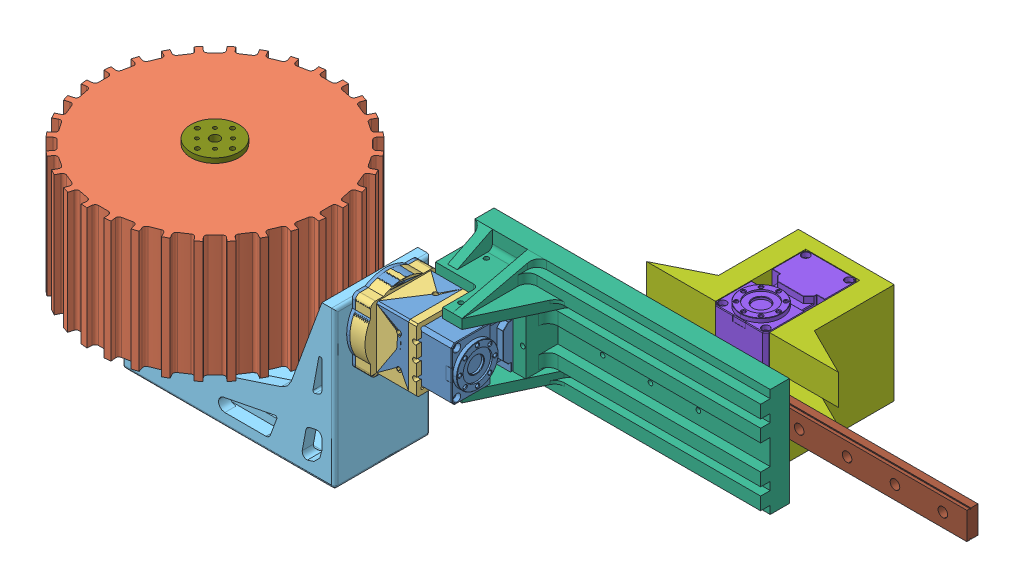
SolidWorks assembly 单轮, configuration Default. Lengths in mm.
Overall size (517.91 123.6 255.15).
20 component instances, 16 part files, 42 mates.
Components (placement in the parent):
- 540总装-1: 540总装 [默认] at (-9.2345 7.2685 42.6291) size (68.75 59.5 48)
- 透明车轮-加工版-1: 透明车轮-加工版 [默认] at (4.5155 78.2685 59.3791) x (0.707107 0 0.707107) z (0 -1 0) size (149.62 149.62 76)
- 3813d-00_asm-2.0-1: 3813d-00_asm-2.0 [默认] at (4.5155 -18.8315 59.3791) x (0.5 0 0.866025) z (0 -1 0)
- 外壳.step-1: 外壳.step [默认] at (-9.2345 51.2685 76.1291) x (0 0 -1) z (0 -1 0) size (48 48 34.5)
- 方案2-大L-1: 方案2-大L [Default] at (39.3905 4.6685 59.3791) x (0 0 -1) z (1 0 0) size (47.8 57 70.75)
- L连接-1: L连接 [Default] at (4.5155 -42.3315 29.3791) x (0 0 1) z (0 1 0) size (60 135 98)
- 540总装-2: 540总装 [默认] at (166.5155 23.5185 73.1291) x (0 0 -1) z (0 1 0) size (68.75 59.5 48)
- 外壳.step-2: 外壳.step [默认] at (122.5155 57.0185 73.1291) x (0 -1 0) z (1 0 0) size (48 48 34.5)
- 新的升降台v4-1: 新的升降台v4 [Default] at (307.5155 6.3685 2.6291) x (0 -1 0) z (0 0 1) size (67.8 185 66)
- 升降-1: 升降 [Default] at (303.824 125.8561 -95.2425) x (0 0 1) z (0 -1 0) size (74.21 120 65.6)
  - 板间外壳-1: 板间外壳 [Default] at (5.2631 83.2739 60.575) size (67 120 63.1)
  - 540舵机-1: 540舵机 [默认] at (58.5131 53.4239 82.575) x (0 -1 0) z (0 0 1) size (33.51 58.5 54.3)
  - 齿轮.step-1: 齿轮.step [默认] at (58.5131 53.4239 115.075) x (0 0 -1) z (-1 0.000114 0) size (8 41.91 41.91)
- HIWIN Corporation-MGW-9C-1: HIWIN Corporation-MGW-9C [Default] at (235.1626 45.0319 -5.4131) x (0 1 0) z (1 0 0) size (30 9.1 39.26)
- HIWIN Corporation-MGWR-9-R0500-1: HIWIN Corporation-MGWR-9-R0500 [Default] at (372.4175 47.7155 -2.8717) x (0 -1 0) z (-1 0 0) size (17 7 120)
- 齿条.step-1: 齿条.step [默认] at (201.2166 22.5685 10.7791) x (1 0 0) z (0 1 0) size (90 11 10)
- 三轴力传感器简易模型-1: 三轴力传感器简易模型 [默认] at (4.5155 -32.3315 59.3791) size (40 20 40)
- 相机固定件改-1: 相机固定件改 [默认] at (47.8155 23.1685 23.7791) x (0 -1 0) z (0 0 -1) size (43 21.7 40.2)
- 相机简易模型-1: 相机简易模型 [默认] at (25.5155 23.1685 21.2791) x (0 -1 0) z (0 0 -1) size (38.4 28.7 38.4)
- 轮子定位件-1: 轮子定位件 [默认] at (4.5155 64.4685 59.3791) x (1 0 0) z (0 1 0) size (30 30 16.8)
Mates (geometry in assembly coordinates):
- 同心1: concentric anti-aligned: cylinder of 540总装-1 through (4.5155 62.7685 59.3791) axis (0 -1 0) radius 16; cylinder of 透明车轮-加工版-1 through (4.5155 2.2685 59.3791) axis (0 1 0) radius 5.05
- 重合1: coincident anti-aligned: plane of 540总装-1 through (4.5155 64.2685 59.3791) normal (0 1 0); plane of 透明车轮-加工版-1 through (4.5155 64.2685 59.3791) normal (0 -1 0)
- 同心2: concentric anti-aligned: cylinder of 540总装-1 through (4.5155 7.3935 59.3791) axis (0 -1 0) radius 5; cylinder of 3813d-00_asm-2.0-1/3813d-00_asm.stp-1/3813D-00_ASM_99_ASM.stp-1/38133-27_40.stp-1 through (4.5155 -17.3315 59.3791) axis (0 1 0) radius 22.5
- 重合5: coincident aligned: plane of 540总装-1 through (-9.2345 51.2685 76.1291) normal (0 -1 0); plane of 外壳.step-1 through (-9.2345 51.2685 76.1291) normal (0 -1 0)
- 同心7: concentric aligned: cylinder of 540总装-1 through (4.5155 7.3935 59.3791) axis (0 -1 0) radius 5; circle of 外壳.step-1
- 同心11: concentric aligned: cylinder of 3813d-00_asm-2.0-1/3813d-00_asm.stp-1/3813D-00_ASM_99_ASM.stp-1/3813D-10_ASM_33_ASM.stp-1/3813D-15_181.stp-1 through (4.5155 -33.3315 59.3791) axis (0 1 0) radius 4.01; cylinder of 方案2-大L-1 through (4.5155 -3.3315 59.3791) axis (0 1 0) radius 4.125
- 同心12: concentric anti-aligned: cylinder of 3813d-00_asm-2.0-1/3813d-00_asm.stp-1/3813D-00_ASM_99_ASM.stp-1/3813D-10_ASM_33_ASM.stp-1/3813D-15_181.stp-1 through (12.5155 -21.7905 45.5227) axis (0 -1 0) radius 1.65; cylinder of 方案2-大L-1 through (12.5155 4.6685 45.5227) axis (0 1 0) radius 2.25
- 重合11: coincident anti-aligned: plane of 3813d-00_asm-2.0-1/3813d-00_asm.stp-1/3813D-00_ASM_99_ASM.stp-1/38133-29_43.stp-1 through (4.5155 -3.3315 59.3791) normal (0 1 0); plane of 方案2-大L-1 through (39.3905 -3.3315 59.3791) normal (0 -1 0)
- 平行4: parallel aligned: plane of 540总装-1 through (49.2655 7.2685 76.1291) normal (1 0 0); plane of 方案2-大L-1 through (53.2655 44.6685 59.3791) normal (1 0 0)
- 同心13: concentric aligned: cylinder of 540总装-1 through (42.5155 37.2685 72.3324) axis (0 0 -1) radius 1.025; cylinder of 方案2-大L-1 through (42.5155 37.2685 80.2791) axis (0 0 -1) radius 1.6
- 同心14: concentric aligned: cylinder of 540总装-1 through (10.5155 37.2685 79.1291) axis (0 0 -1) radius 1.5; cylinder of 外壳.step-1 through (10.5155 37.2685 79.1291) axis (0 0 -1) radius 1.5
- 同心15: concentric aligned: cylinder of 3813d-00_asm-2.0-1/3813d-00_asm.stp-1/3813D-00_ASM_99_ASM.stp-1/3813D-10_ASM_33_ASM.stp-1/3813D-15_181.stp-1 through (9.0155 -33.3315 67.1733) axis (0 1 0) radius 1.51; cylinder of 方案2-大L-1 through (-0.4845 -3.3315 64.3791) axis (0 1 0) radius 1.6
- 同心16: concentric aligned: cylinder of 3813d-00_asm-2.0-1/3813d-00_asm.stp-1/3813D-00_ASM_99_ASM.stp-1/3813D-26_48.stp-1 through (4.5155 -20.3315 59.3791) axis (0 -1 0) radius 22.5; cylinder of L连接-1 through (4.5155 -34.3315 59.3791) axis (0 -1 0) radius 30
- 重合12: coincident anti-aligned: plane of 3813d-00_asm-2.0-1/3813d-00_asm.stp-1/3813D-00_ASM_99_ASM.stp-1/38133-29_43.stp-2 through (4.5155 -34.3315 59.3791) normal (0 -1 0); plane of L连接-1 through (4.5155 -34.3315 29.3791) normal (0 1 0)
- 同心17: concentric anti-aligned: cylinder of 3813d-00_asm-2.0-1/3813d-00_asm.stp-1/3813D-00_ASM_99_ASM.stp-1/3813D-10_ASM_33_ASM.stp-1/3813D-15_181.stp-1 through (9.0155 -33.3315 67.1733) axis (0 1 0) radius 1.51; cylinder of L连接-1 through (9.0155 -34.3315 67.1733) axis (0 -1 0) radius 1.625
- 同心18: concentric aligned: cylinder of 540总装-2 through (109.5155 40.2685 59.3791) axis (1 0 0) radius 15; cylinder of 外壳.step-2 through (112.5155 40.2685 59.3791) axis (1 0 0) radius 14
- 重合13: coincident anti-aligned: plane of 540总装-2 through (122.5155 40.2685 59.3791) normal (-1 0 0); plane of 外壳.step-2 through (122.5155 57.0185 73.1291) normal (1 0 0)
- 同心19: concentric aligned: cylinder of 540总装-2 through (136.5155 30.2685 73.1291) axis (0 0 1) radius 1.5; cylinder of 外壳.step-2 through (136.5155 30.2685 73.1291) axis (0 0 1) radius 1.5
- 重合14: coincident anti-aligned: plane of L连接-1 through (109.5155 -34.3315 29.3791) normal (1 0 0); plane of 540总装-2 through (109.5155 40.2685 59.3791) normal (-1 0 0)
- 同心22: concentric anti-aligned: cylinder of L连接-1 through (39.5155 40.2685 59.3791) axis (1 0 0) radius 1.6; cylinder of 540总装-2 through (109.5155 40.2685 59.3791) axis (-1 0 0) radius 1.25
- 重合16: coincident anti-aligned: plane of 540总装-2 through (166.5155 57.0185 14.6291) normal (0 0 -1); plane of 新的升降台v4-1 through (307.5155 6.3685 14.6291) normal (0 0 1)
- 同心23: concentric anti-aligned: cylinder of 540总装-2 through (136.5155 50.2685 18.4258) axis (0 0 -1) radius 1.025; cylinder of 新的升降台v4-1 through (136.5155 50.2685 -1.4721) axis (0 0 1) radius 1.45
- 同心24: concentric anti-aligned: cylinder of 540总装-2 through (136.5155 30.2685 18.4258) axis (0 0 -1) radius 1.025; cylinder of 新的升降台v4-1 through (136.5155 30.2685 -1.4721) axis (0 0 1) radius 1.45
- 平行6: parallel aligned: plane of 新的升降台v4-1 through (307.5155 6.3685 2.6291) normal (0 0 -1); plane of L连接-1 through (4.5155 -34.3315 29.3791) normal (0 0 -1)
- 平行7: parallel anti-aligned: plane of 新的升降台v4-1 through (307.5155 6.3685 2.6291) normal (0 0 -1); plane of 升降-1/板间外壳-1 through (220.5501 21.1811 -24.9794) normal (0 0 1)
- 平行8: parallel aligned: plane of 新的升降台v4-1 through (307.5155 6.3685 14.6291) normal (1 0 0); plane of 升降-1/板间外壳-1 through (280.5501 21.1811 -89.9794) normal (1 0 0)
- 同心27: concentric anti-aligned: cylinder of HIWIN Corporation-MGW-9C-1 through (265.2255 39.4155 -1.5709) axis (-1 0 0) radius 0.35; cylinder of HIWIN Corporation-MGWR-9-R0500-1 through (122.4175 39.4155 -1.5709) axis (1 0 0) radius 0.35
- 重合20: coincident anti-aligned: plane of 新的升降台v4-1 through (307.5155 6.3685 10.7791) normal (0 0 -1); plane of 齿条.step-1 through (201.2166 12.5685 10.7791) normal (0 0 1)
- 重合22: coincident anti-aligned: plane of 新的升降台v4-1 through (307.5155 12.5685 10.7791) normal (0 1 0); plane of 齿条.step-1 through (201.2166 12.5685 -0.2209) normal (0 -1 0)
- 重合28: coincident anti-aligned: plane of 方案2-大L-1 through (27.5155 49.2689 45.4791) normal (-1 0 0); plane of 相机固定件改-1 through (27.5155 51.2343 45.2791) normal (1 0 0)
- 重合29: coincident aligned: plane of 方案2-大L-1 through (39.3905 44.6685 59.3791) normal (0 1 0); plane of 相机固定件改-1 through (23.8155 44.6685 2.2791) normal (0 1 0)
- 重合30: coincident aligned: plane of 方案2-大L-1 through (39.3905 44.6685 42.4791) normal (0 0 1); plane of 相机固定件改-1 through (33.8155 47.084 42.4791) normal (0 0 1)
- 重合31: coincident anti-aligned: plane of 相机固定件改-1 through (25.5155 23.1685 23.7791) normal (-1 0 0); plane of 相机简易模型-1 through (25.5155 23.1685 21.2791) normal (1 0 0)
- 同心29: concentric anti-aligned: circle of 相机固定件改-1; circle of 相机简易模型-1
- 平行13: parallel aligned: plane of 相机固定件改-1 through (23.8155 44.6685 2.2791) normal (0 0 -1); plane of 相机简易模型-1 through (23.8155 42.3685 2.0791) normal (0 0 -1)
- 同心30: concentric aligned: cylinder of 方案2-大L-1 through (-0.4845 -3.3315 54.3791) axis (0 1 0) radius 1.6; circle of 三轴力传感器简易模型-1
- 平行14: parallel aligned: plane of 方案2-大L-1 through (39.3905 4.6685 35.4791) normal (0 0 -1); plane of 三轴力传感器简易模型-1 through (-15.4845 -12.3315 39.3791) normal (0 0 -1)
- 重合33: coincident anti-aligned: plane of L连接-1 through (4.5155 -32.3315 29.3791) normal (0 1 0); plane of 三轴力传感器简易模型-1 through (4.5155 -32.3315 59.3791) normal (0 -1 0)
- 同心31: concentric anti-aligned: cylinder of 540总装-1 through (4.5155 64.2685 48.3791) axis (0 1 0) radius 1.45; cylinder of 透明车轮-加工版-1 through (4.5155 78.2685 48.3791) axis (0 -1 0) radius 1.45
- 重合34: coincident anti-aligned: plane of 透明车轮-加工版-1 through (4.5155 78.2685 59.3791) normal (0 1 0); plane of 轮子定位件-1 through (4.5155 78.2685 59.3791) normal (0 -1 0)
- 同心32: concentric aligned: cylinder of 透明车轮-加工版-1 through (4.5155 2.2685 59.3791) axis (0 1 0) radius 5.05; cylinder of 轮子定位件-1 through (4.5155 71.2685 59.3791) axis (0 1 0) radius 3
- 同心33: concentric aligned: cylinder of 透明车轮-加工版-1 through (4.5155 78.2685 48.3791) axis (0 -1 0) radius 1.45; cylinder of 轮子定位件-1 through (4.5155 81.2685 48.3791) axis (0 -1 0) radius 1.4
